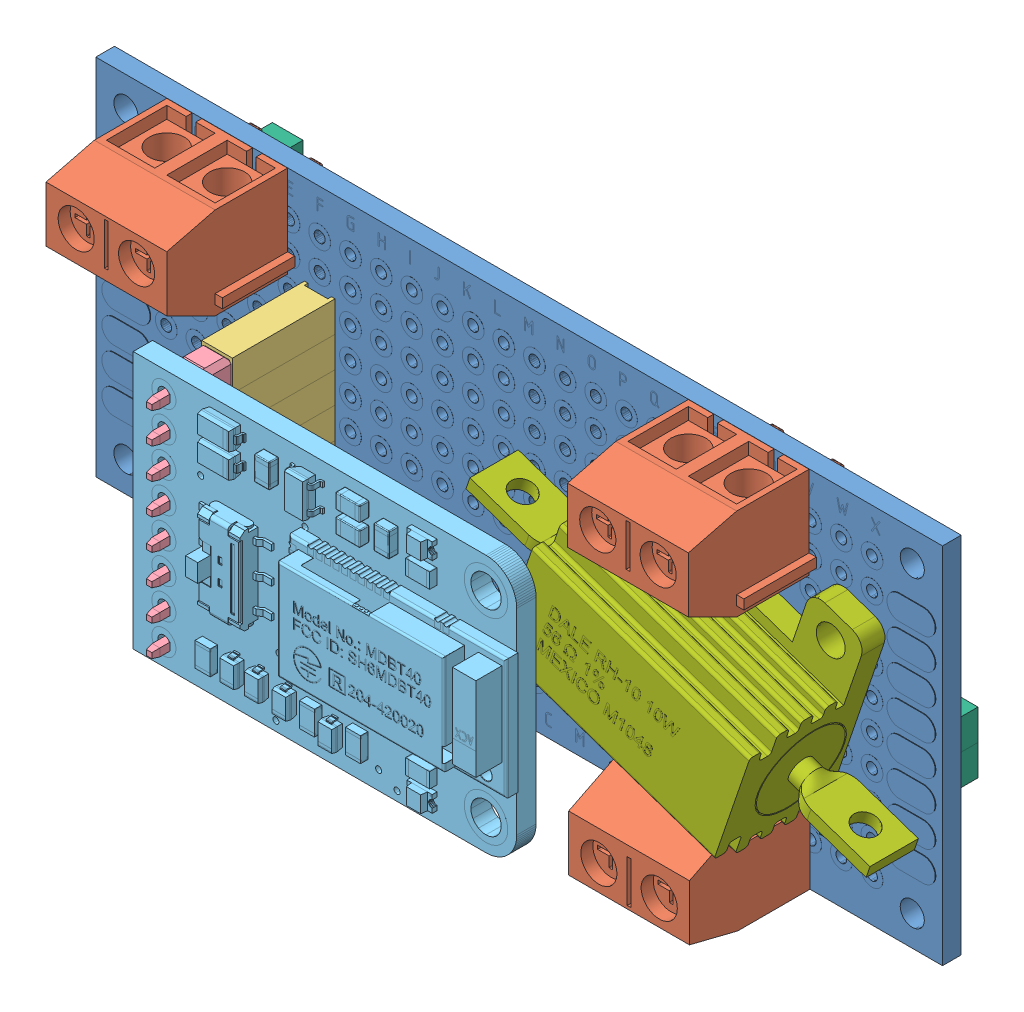
SolidWorks assembly BLEShunt, configuration Default. Lengths in mm.
Overall size (73.24 30.62 25.87).
19 component instances, 7 part files, 42 mates.
Components (placement in the parent):
- 3x7PerfBoard-1: 3x7PerfBoard [Default] at origin size (70.1 30.1 1.65)
- 5mm2PTerminalBlock-1: 5mm2PTerminalBlock [Default] at (-19.17 15.03 1.55) x (-1 0 0) z (0 0 1) size (10.6 7.6 15)
- FemalePinHeader8By1.stp-1: FemalePinHeader8By1.stp [Default] at (-16.51 6.35 1.55) x (0 -1 0) z (0 0 1) size (20.32 2.54 11.7)
  - Female Pin Header 1x.stp-1: Female Pin Header 1x.stp [Default] at origin size (2.54 2.54 11.7)
  - Female Pin Header 1x.stp-2: Female Pin Header 1x.stp [Default] at (2.54 0 0) size (2.54 2.54 11.7)
  - Female Pin Header 1x.stp-3: Female Pin Header 1x.stp [Default] at (5.08 0 0) size (2.54 2.54 11.7)
  - Female Pin Header 1x.stp-4: Female Pin Header 1x.stp [Default] at (7.62 0 0) size (2.54 2.54 11.7)
  - Female Pin Header 1x.stp-5: Female Pin Header 1x.stp [Default] at (10.16 0 0) size (2.54 2.54 11.7)
  - Female Pin Header 1x.stp-6: Female Pin Header 1x.stp [Default] at (12.7 0 0) size (2.54 2.54 11.7)
  - Female Pin Header 1x.stp-7: Female Pin Header 1x.stp [Default] at (15.24 0 0) size (2.54 2.54 11.7)
  - Female Pin Header 1x.stp-8: Female Pin Header 1x.stp [Default] at (17.78 0 0) size (2.54 2.54 11.7)
- 1x8 Male Pin Header.step-1: 1x8 Male Pin Header.step [Default] at (-16.59 6.27 12.59) x (0 -1 0) z (1 0 0) size (20.32 13.54 2.5)
- BLEFriend.stp-1: BLEFriend.stp [Default] at (-19.31 8.128 12.59) x (0 -1 0) z (0 0 1) size (21.35 31.87 4.78)
- 5mm2PTerminalBlock-2: 5mm2PTerminalBlock [Default] at (24.01 15.03 1.55) x (-1 0 0) z (0 0 1) size (10.6 7.6 15)
- 5mm2PTerminalBlock-5: 5mm2PTerminalBlock [Default] at (14.1 -15.03 1.55) size (10.6 7.6 15)
- FemalePinHeader2By1-1: FemalePinHeader2By1 [Default] at (-29.21 -8.89 0) x (0 -1 0) z (0 0 -1) size (5.08 2.54 11.7)
- FemalePinHeader2By1-2: FemalePinHeader2By1 [Default] at (-29.21 6.35 0) x (0 -1 0) z (0 0 -1) size (5.08 2.54 11.7)
- FemalePinHeader2By1-3: FemalePinHeader2By1 [Default] at (26.67 -6.35 0) x (0 -1 0) z (0 0 -1) size (5.08 2.54 11.7)
- ShuntResistor-1: ShuntResistor [Default<As Machined>] at (18.3281 0.2483 1.55) x (0.946299 -0.323291 0) z (-0.323291 -0.946299 0) size (35 9.71 20.4)
Mates (geometry in assembly coordinates):
- Coincident1: coincident aligned: plane of 3x7PerfBoard-1 through (0 0 0) normal (0 0 1)
- Coincident2: coincident aligned: plane of 3x7PerfBoard-1 through (0 0 0) normal (0 1 0)
- Coincident3: coincident aligned: plane of 3x7PerfBoard-1 through (0 0 0) normal (1 0 0)
- Parallel1: parallel aligned: plane of 3x7PerfBoard-1 through (-35.05 15.05 0) normal (0 1 0); plane of 5mm2PTerminalBlock-1 through (-19.17 15.03 1.55) normal (0 1 0)
- Width1: width: cylinder of 5mm2PTerminalBlock-1; plane of 3x7PerfBoard-1 through (-26.27 11.93 -3.45) normal (1 0 0); cylinder of 5mm2PTerminalBlock-1 through (-26.67 11.43 0) axis (0 0 -1) radius 0.45
- Width2: width: plane of 5mm2PTerminalBlock-1 through (-21.27 11.93 -3.45) normal (0 1 0); plane of 3x7PerfBoard-1 through (-21.27 10.93 -3.45) normal (0 -1 0); cylinder of 5mm2PTerminalBlock-1 through (-26.67 11.43 0) axis (0 0 -1) radius 0.45
- Coincident5: coincident anti-aligned: plane of 3x7PerfBoard-1 through (0 0 1.55) normal (0 0 1); plane of 5mm2PTerminalBlock-1 through (-19.17 15.03 1.55) normal (0 0 -1)
- Parallel2: parallel aligned: plane of 3x7PerfBoard-1 through (35.05 -15.05 0) normal (0 -1 0); plane of FemalePinHeader8By1.stp-1/Female Pin Header 1x.stp-8 through (-17.78 -12.7 1.55) normal (0 -1 0)
- Coincident7: coincident anti-aligned: plane of 3x7PerfBoard-1 through (0 0 1.55) normal (0 0 1); plane of FemalePinHeader8By1.stp-1/Female Pin Header 1x.stp-8 through (-16.51 -11.43 1.55) normal (0 0 -1)
- Width3: width: plane of FemalePinHeader8By1.stp-1/Female Pin Header 1x.stp-8 through (-16.31 -12.53 1.55) normal (1 0 0); plane of 3x7PerfBoard-1 through (-16.71 -10.33 1.55) normal (-1 0 0); cylinder of FemalePinHeader8By1.stp-1/Female Pin Header 1x.stp-8 through (-16.51 -11.43 0) axis (0 0 -1) radius 0.45
- Width4: width: plane of FemalePinHeader8By1.stp-1/Female Pin Header 1x.stp-8 through (-16.71 -11.755 -1.65) normal (0 -1 0); plane of 3x7PerfBoard-1 through (-16.71 -11.105 2.35) normal (0 1 0); cylinder of FemalePinHeader8By1.stp-1/Female Pin Header 1x.stp-8 through (-16.51 -11.43 0) axis (0 0 -1) radius 0.45
- Coincident8: coincident anti-aligned: plane of FemalePinHeader8By1.stp-1/Female Pin Header 1x.stp-7 through (-16.51 -8.89 10.05) normal (0 0 1); plane of 1x8 Male Pin Header.step-1 through (-16.59 -3.89 10.05) normal (0 0 -1)
- Coincident9: coincident anti-aligned: plane of FemalePinHeader8By1.stp-1/Female Pin Header 1x.stp-8 through (-16.11 -11.83 10.05) normal (0 1 0); plane of 1x8 Male Pin Header.step-1 through (-16.27 -11.83 2.05) normal (0 -1 0)
- Coincident10: coincident anti-aligned: plane of FemalePinHeader8By1.stp-1/Female Pin Header 1x.stp-8 through (-16.91 -11.83 10.05) normal (1 0 0); plane of 1x8 Male Pin Header.step-1 through (-16.91 -11.19 2.05) normal (-1 0 0)
- Coincident11: coincident anti-aligned: plane of 1x8 Male Pin Header.step-1 through (-16.59 6.27 12.59) normal (0 0 1); plane of BLEFriend.stp-1 through (12.44 8.128 12.59) normal (0 0 -1)
- Tangent1: tangent: plane of 1x8 Male Pin Header.step-1 through (-16.27 -11.19 2.05) normal (1 0 0); curve of BLEFriend.stp-1
- Tangent2: tangent: plane of 1x8 Male Pin Header.step-1 through (-16.27 6.59 2.05) normal (1 0 0); curve of BLEFriend.stp-1
- Symmetric1: symmetric aligned: plane of FemalePinHeader8By1.stp-1/Female Pin Header 1x.stp-4 through (-17.78 -2.54 1.55) normal (0 -1 0); plane of BLEFriend.stp-1 through (9.9 8.128 14.19) normal (0 1 0); plane of BLEFriend.stp-1 through (9.9 -13.208 12.59) normal (0 -1 0)
- Width5: width: plane of 5mm2PTerminalBlock-2 through (16.11 11.93 -3.45) normal (-1 0 0); plane of 3x7PerfBoard-1 through (16.91 11.93 -3.45) normal (1 0 0); cylinder of 5mm2PTerminalBlock-2 through (16.51 11.43 0) axis (0 0 -1) radius 0.45
- Width6: width: plane of 5mm2PTerminalBlock-2 through (21.91 11.93 -3.45) normal (0 1 0); plane of 3x7PerfBoard-1 through (21.91 10.93 -3.45) normal (0 -1 0); cylinder of 5mm2PTerminalBlock-2 through (16.52 11.43 -0.005) axis (0 0 -1) radius 0.45
- Coincident12: coincident anti-aligned: plane of 3x7PerfBoard-1 through (0 0 1.55) normal (0 0 1); plane of 5mm2PTerminalBlock-2 through (24.01 15.03 1.55) normal (0 0 -1)
- Parallel3: parallel aligned: plane of 3x7PerfBoard-1 through (-35.05 15.05 0) normal (0 1 0); plane of 5mm2PTerminalBlock-2 through (24.01 15.03 1.55) normal (0 1 0)
- Parallel6: parallel aligned: plane of 3x7PerfBoard-1 through (35.05 -15.05 0) normal (0 -1 0); plane of 5mm2PTerminalBlock-5 through (14.1 -15.03 1.55) normal (0 -1 0)
- Coincident14: coincident anti-aligned: plane of 3x7PerfBoard-1 through (0 0 1.55) normal (0 0 1); plane of 5mm2PTerminalBlock-5 through (14.1 -15.03 1.55) normal (0 0 -1)
- Width10: width: plane of 5mm2PTerminalBlock-5 through (16.2 -11.93 -3.45) normal (0 -1 0); plane of 3x7PerfBoard-1 through (16.2 -10.93 -3.45) normal (0 1 0); cylinder of 5mm2PTerminalBlock-5 through (29.21 -11.43 0) axis (0 0 -1) radius 0.45
- Width11: width: plane of 5mm2PTerminalBlock-5 through (22 -11.93 -3.45) normal (1 0 0); plane of 3x7PerfBoard-1 through (21.2 -11.93 -3.45) normal (-1 0 0); cylinder of 5mm2PTerminalBlock-5 through (21.6 -11.43 -0.005) axis (0 0 -1) radius 0.45
- Coincident15: coincident anti-aligned: plane of 3x7PerfBoard-1 through (0 0 0) normal (0 0 -1); plane of FemalePinHeader2By1-1 through (-29.21 -8.89 0) normal (0 0 1)
- Width12: width: plane of FemalePinHeader2By1-1 through (-29.01 -10.33 0) normal (1 0 0); plane of FemalePinHeader2By1-1 through (-29.41 -12.53 0) normal (-1 0 0); cylinder of 3x7PerfBoard-1 through (-29.21 -11.43 -0.005) axis (0 0 -1) radius 0.45
- Width13: width: plane of FemalePinHeader2By1-1 through (-29.01 -11.755 3.2) normal (0 -1 0); plane of FemalePinHeader2By1-1 through (-29.01 -11.105 -0.8) normal (0 1 0); cylinder of 3x7PerfBoard-1 through (-29.21 -11.43 -0.005) axis (0 0 -1) radius 0.45
- Parallel7: parallel aligned: plane of 3x7PerfBoard-1 through (35.05 -15.05 0) normal (0 -1 0); plane of FemalePinHeader2By1-1 through (-27.94 -12.7 0) normal (0 -1 0)
- Coincident17: coincident anti-aligned: plane of 3x7PerfBoard-1 through (0 0 0) normal (0 0 -1); plane of FemalePinHeader2By1-2 through (-29.21 6.35 0) normal (0 0 1)
- Parallel8: parallel aligned: plane of 3x7PerfBoard-1 through (35.05 -15.05 0) normal (0 -1 0); plane of FemalePinHeader2By1-2 through (-27.94 2.54 0) normal (0 -1 0)
- Width15: width: plane of FemalePinHeader2By1-2 through (-29.01 4.91 0) normal (1 0 0); plane of FemalePinHeader2By1-2 through (-29.41 2.71 0) normal (-1 0 0); cylinder of 3x7PerfBoard-1 through (-29.21 -11.43 -0.005) axis (0 0 -1) radius 0.45
- Width16: width: plane of FemalePinHeader2By1-2 through (-29.01 3.485 3.2) normal (0 -1 0); plane of FemalePinHeader2By1-2 through (-29.01 4.135 -0.8) normal (0 1 0); cylinder of 3x7PerfBoard-1 through (-29.21 3.81 0) axis (0 0 -1) radius 0.45
- Coincident18: coincident anti-aligned: plane of 3x7PerfBoard-1 through (0 0 0) normal (0 0 -1); plane of FemalePinHeader2By1-3 through (26.67 -8.89 0) normal (0 0 1)
- Parallel9: parallel aligned: plane of 3x7PerfBoard-1 through (35.05 -15.05 0) normal (0 -1 0); plane of FemalePinHeader2By1-3 through (27.94 -12.7 0) normal (0 -1 0)
- Width18: width: plane of FemalePinHeader2By1-3 through (26.87 -9.215 3.2) normal (0 -1 0); plane of FemalePinHeader2By1-3 through (26.87 -8.565 -0.8) normal (0 1 0); cylinder of 3x7PerfBoard-1 through (26.68 -8.89 -0.005) axis (0 0 -1) radius 0.45
- Width19: width: plane of FemalePinHeader2By1-3 through (26.87 -10.33 0) normal (1 0 0); plane of FemalePinHeader2By1-3 through (26.47 -12.53 0) normal (-1 0 0); cylinder of 3x7PerfBoard-1 through (26.67 -11.43 0) axis (0 0 -1) radius 0.45
- Coincident19: coincident anti-aligned: plane of 3x7PerfBoard-1 through (0 0 1.55) normal (0 0 1); plane of ShuntResistor-1 through (26.8209 6.8576 1.55) normal (0 0 -1)
- Coincident20: coincident: line of 5mm2PTerminalBlock-2 through (14.01 7.43 1.55) axis (0 0 1); plane of ShuntResistor-1 through (11.084 8.4296 3.45) normal (0.323291 0.946299 0)
- Coincident21: coincident: line of 5mm2PTerminalBlock-5 through (24.1 -7.43 1.55) axis (0 0 1); plane of ShuntResistor-1 through (12.1347 -3.3422 3.45) normal (-0.323291 -0.946299 0)
- Coincident22: coincident: plane of 3x7PerfBoard-1 through (35.05 15.05 0) normal (1 0 0); line of ShuntResistor-1 through (35.05 -4.9361 7.55) axis (0 0 -1)
